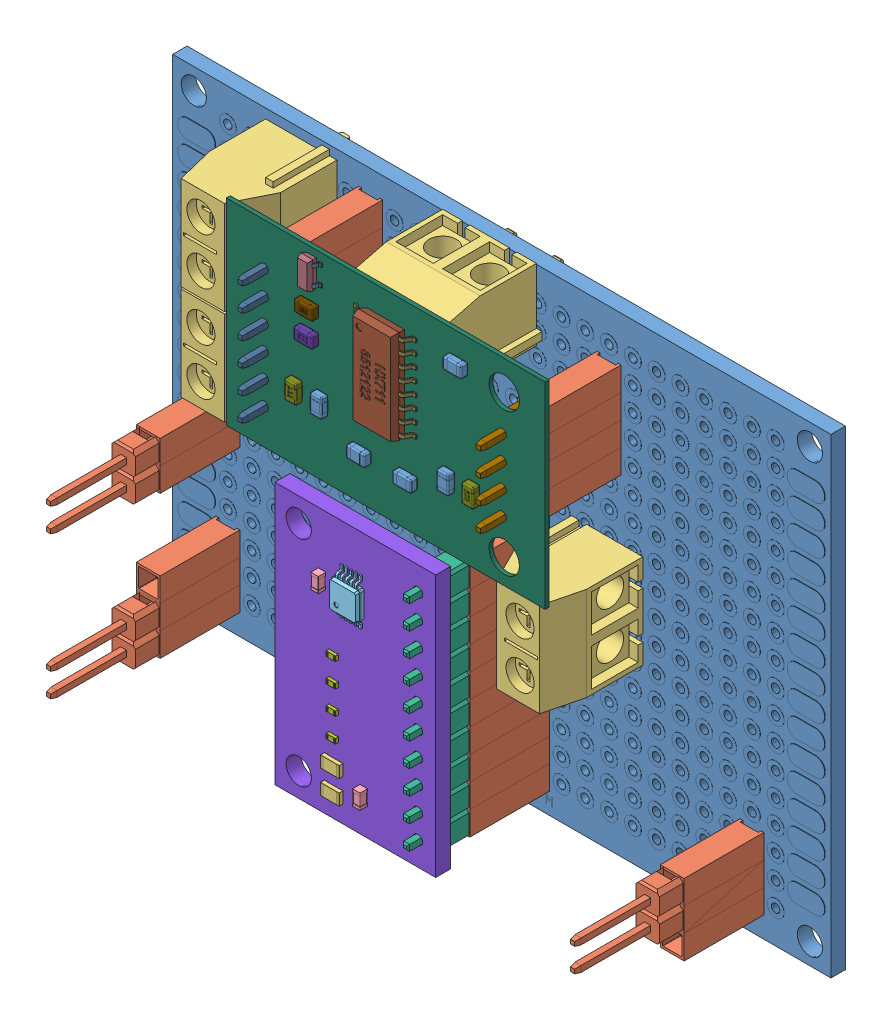
SolidWorks assembly ADCPCB, configuration Default. Lengths in mm.
Overall size (70.2 51.25 24.04).
104 component instances, 21 part files, 65 mates.
Components (placement in the parent):
- 5x7PCBBoard.stp-1: 5x7PCBBoard.stp [Default] at origin size (70.2 50.2 1.66)
- FemalePinHeader2By1.stp-1: FemalePinHeader2By1.stp [Default] at (-29.21 -21.59 1.54) x (0 1 0) z (0 0 1) size (5.08 2.54 11.7)
  - Female Pin Header 1x.stp-1: Female Pin Header 1x.stp [Default] at origin size (2.54 2.54 11.7)
  - Female Pin Header 1x.stp-2: Female Pin Header 1x.stp [Default] at (2.54 0 0) size (2.54 2.54 11.7)
- FemalePinHeader2By1.stp-2: FemalePinHeader2By1.stp [Default] at (-29.21 -6.35 1.54) x (0 1 0) z (0 0 1) size (5.08 2.54 11.7)
  - Female Pin Header 1x.stp-1: Female Pin Header 1x.stp [Default] at origin size (2.54 2.54 11.7)
  - Female Pin Header 1x.stp-2: Female Pin Header 1x.stp [Default] at (2.54 0 0) size (2.54 2.54 11.7)
- FemalePinHeader2By1.stp-3: FemalePinHeader2By1.stp [Default] at (-29.21 -19.05 1.54) x (0 1 0) z (0 0 1) size (5.08 2.54 11.7)
  - Female Pin Header 1x.stp-1: Female Pin Header 1x.stp [Default] at origin size (2.54 2.54 11.7)
  - Female Pin Header 1x.stp-2: Female Pin Header 1x.stp [Default] at (2.54 0 0) size (2.54 2.54 11.7)
- FemalePinHeader2By1.stp-4: FemalePinHeader2By1.stp [Default] at (26.67 -21.59 1.54) x (0 1 0) z (0 0 1) size (5.08 2.54 11.7)
  - Female Pin Header 1x.stp-1: Female Pin Header 1x.stp [Default] at origin size (2.54 2.54 11.7)
  - Female Pin Header 1x.stp-2: Female Pin Header 1x.stp [Default] at (2.54 0 0) size (2.54 2.54 11.7)
- FemalePinHeader2By1.stp-5: FemalePinHeader2By1.stp [Default] at (26.67 -19.05 1.54) x (0 1 0) z (0 0 1) size (5.08 2.54 11.7)
  - Female Pin Header 1x.stp-1: Female Pin Header 1x.stp [Default] at origin size (2.54 2.54 11.7)
  - Female Pin Header 1x.stp-2: Female Pin Header 1x.stp [Default] at (2.54 0 0) size (2.54 2.54 11.7)
- FemalePinHeader10By1.stp-1: FemalePinHeader10By1.stp [Default] at (3.81 1.27 1.54) x (0 -1 0) z (0 0 1) size (25.4 2.54 11.7)
  - Female Pin Header 1x.stp-1: Female Pin Header 1x.stp [Default] at origin size (2.54 2.54 11.7)
  - Female Pin Header 1x.stp-2: Female Pin Header 1x.stp [Default] at (2.54 0 0) size (2.54 2.54 11.7)
  - Female Pin Header 1x.stp-3: Female Pin Header 1x.stp [Default] at (5.08 0 0) size (2.54 2.54 11.7)
  - Female Pin Header 1x.stp-4: Female Pin Header 1x.stp [Default] at (7.62 0 0) size (2.54 2.54 11.7)
  - Female Pin Header 1x.stp-5: Female Pin Header 1x.stp [Default] at (10.16 0 0) size (2.54 2.54 11.7)
  - Female Pin Header 1x.stp-6: Female Pin Header 1x.stp [Default] at (12.7 0 0) size (2.54 2.54 11.7)
  - Female Pin Header 1x.stp-7: Female Pin Header 1x.stp [Default] at (15.24 0 0) size (2.54 2.54 11.7)
  - Female Pin Header 1x.stp-8: Female Pin Header 1x.stp [Default] at (17.78 0 0) size (2.54 2.54 11.7)
  - Female Pin Header 1x.stp-9: Female Pin Header 1x.stp [Default] at (20.32 0 0) size (2.54 2.54 11.7)
  - Female Pin Header 1x.stp-10: Female Pin Header 1x.stp [Default] at (22.86 0 0) size (2.54 2.54 11.7)
- FemalePinHeader6By1.stp-1: FemalePinHeader6By1.stp [Default] at (-13.97 21.59 1.54) x (0 -1 0) z (0 0 1) size (15.24 2.54 11.7)
  - Female Pin Header 1x.stp-1: Female Pin Header 1x.stp [Default] at origin size (2.54 2.54 11.7)
  - Female Pin Header 1x.stp-2: Female Pin Header 1x.stp [Default] at (2.54 0 0) size (2.54 2.54 11.7)
  - Female Pin Header 1x.stp-3: Female Pin Header 1x.stp [Default] at (5.08 0 0) size (2.54 2.54 11.7)
  - Female Pin Header 1x.stp-4: Female Pin Header 1x.stp [Default] at (7.62 0 0) size (2.54 2.54 11.7)
  - Female Pin Header 1x.stp-5: Female Pin Header 1x.stp [Default] at (10.16 0 0) size (2.54 2.54 11.7)
  - Female Pin Header 1x.stp-6: Female Pin Header 1x.stp [Default] at (12.7 0 0) size (2.54 2.54 11.7)
- FemalePinHeader4By1.stp-1: FemalePinHeader4By1.stp [Default] at (11.44 19.05 1.54) x (0 -1 0) z (0 0 1) size (10.16 2.54 11.7)
  - Female Pin Header 1x.stp-1: Female Pin Header 1x.stp [Default] at origin size (2.54 2.54 11.7)
  - Female Pin Header 1x.stp-2: Female Pin Header 1x.stp [Default] at (2.54 0 0) size (2.54 2.54 11.7)
  - Female Pin Header 1x.stp-3: Female Pin Header 1x.stp [Default] at (5.08 0 0) size (2.54 2.54 11.7)
  - Female Pin Header 1x.stp-4: Female Pin Header 1x.stp [Default] at (7.62 0 0) size (2.54 2.54 11.7)
- ADS1115+PinHeader.step-1: ADS1115+PinHeader.step [Default] at (144.065 -99.14 12.63) x (-1 0 0) z (0 0 1) size (17.14 27.94 11.54)
  - R_0805_2012Metric.step-1: R_0805_2012Metric.step [Default] at (149.225 -80.01 1.65) size (2 1.2 0.45)
    - SOLID.step-1: SOLID.step [Default] at origin size (2 1.2 0.45)
  - R_0805_2012Metric.step-2: R_0805_2012Metric.step [Default] at (149.225 -77.47 1.65) size (2 1.2 0.45)
    - SOLID.step-1: SOLID.step [Default] at origin size (2 1.2 0.45)
  - C_0603_1608Metric.step-1: C_0603_1608Metric.step [Default] at (150.495 -96.52 1.65) x (0 1 0) z (0 0 1) size (1.6 0.8 0.8)
    - SOLID-0.step-1: SOLID-0.step [Default] at origin size (1.6 0.8 0.8)
  - TSSOP-10_3x3mm_P0.5mm.step-1: TSSOP-10_3x3mm_P0.5mm.step [Default] at (147.32 -96.52 1.65) x (0 -1 0) z (0 0 1) size (4.9 3 1)
    - SOLID-1.step-1: SOLID-1.step [Default] at origin size (4.9 3 1)
  - PinHeader_1x10_P2.54mm_Vertical.step-1: PinHeader_1x10_P2.54mm_Vertical.step [Default] at (140.335 -77.47 -0.05) x (-1 0 0) z (0 0 -1) size (2.54 25.4 11.54)
    - SOLID-2.step-1: SOLID-2.step [Default] at origin size (2.54 25.4 11.54)
  - C_0603_1608Metric.step-2: C_0603_1608Metric.step [Default] at (146.05 -78.74 1.65) x (0 1 0) z (0 0 1) size (1.6 0.8 0.8)
    - SOLID-0.step-1: SOLID-0.step [Default] at origin size (1.6 0.8 0.8)
  - R_0402_1005Metric.step-1: R_0402_1005Metric.step [Default] at (149.225 -85.09 1.65) x (-1 0 0) z (0 0 1) size (1 0.5 0.35)
    - SOLID-3.step-1: SOLID-3.step [Default] at origin size (1 0.5 0.35)
  - R_0402_1005Metric.step-2: R_0402_1005Metric.step [Default] at (149.225 -82.55 1.65) x (-1 0 0) z (0 0 1) size (1 0.5 0.35)
    - SOLID-3.step-1: SOLID-3.step [Default] at origin size (1 0.5 0.35)
  - R_0402_1005Metric.step-3: R_0402_1005Metric.step [Default] at (149.225 -87.63 1.65) size (1 0.5 0.35)
    - SOLID-3.step-1: SOLID-3.step [Default] at origin size (1 0.5 0.35)
  - R_0402_1005Metric.step-4: R_0402_1005Metric.step [Default] at (149.225 -90.17 1.65) x (-1 0 0) z (0 0 1) size (1 0.5 0.35)
    - SOLID-3.step-1: SOLID-3.step [Default] at origin size (1 0.5 0.35)
  - COMPOUND.step-1: COMPOUND.step [Default] at origin size (17.14 27.94 1.6)
- 1x4 Male Pin Header.step-1: 1x4 Male Pin Header.step [Default] at (11.52 11.51 12.58) x (0 1 0) z (-1 0 0) size (10.17 13.54 2.5)
- 1x6 Male Pin Header.step-1: 1x6 Male Pin Header.step [Default] at (-13.89 8.97 12.58) x (0 1 0) z (-1 0 0) size (15.24 13.54 2.5)
- HX711.STEP-1: HX711.STEP [Default] at (-17.9207 5.1545 12.58) size (34 21 1.97)
  - HX711_SOP16_Valor predeterminado.STEP-1: HX711_SOP16_Valor predeterminado.STEP [Default] at (16.3915 14.4374 -9.5535) size (6.7 10 1.56)
    - base_HX711_Valor predeterminado.STEP-1: base_HX711_Valor predeterminado.STEP [Default] at (0.6189 -0.8581 10) size (4.4 10 1.52)
    - pino_HX711_Valor predeterminado.STEP-1: pino_HX711_Valor predeterminado.STEP [Default] at (-2.7311 3.5869 10.04) x (0 -1 0) z (-1 0 0) size (0.4 0.86 1.3)
    - pino_HX711_Valor predeterminado.STEP-2: pino_HX711_Valor predeterminado.STEP [Default] at (-2.7311 2.3169 10.04) x (0 -1 0) z (-1 0 0) size (0.4 0.86 1.3)
    - pino_HX711_Valor predeterminado.STEP-3: pino_HX711_Valor predeterminado.STEP [Default] at (-2.7311 1.0469 10.04) x (0 -1 0) z (-1 0 0) size (0.4 0.86 1.3)
    - pino_HX711_Valor predeterminado.STEP-4: pino_HX711_Valor predeterminado.STEP [Default] at (-2.7311 -0.2231 10.04) x (0 -1 0) z (-1 0 0) size (0.4 0.86 1.3)
    - pino_HX711_Valor predeterminado.STEP-5: pino_HX711_Valor predeterminado.STEP [Default] at (-2.7311 -1.4931 10.04) x (0 -1 0) z (-1 0 0) size (0.4 0.86 1.3)
    - pino_HX711_Valor predeterminado.STEP-6: pino_HX711_Valor predeterminado.STEP [Default] at (-2.7311 -2.7631 10.04) x (0 -1 0) z (-1 0 0) size (0.4 0.86 1.3)
    - pino_HX711_Valor predeterminado.STEP-7: pino_HX711_Valor predeterminado.STEP [Default] at (-2.7311 -4.0331 10.04) x (0 -1 0) z (-1 0 0) size (0.4 0.86 1.3)
    - pino_HX711_Valor predeterminado.STEP-8: pino_HX711_Valor predeterminado.STEP [Default] at (-2.7311 -5.3031 10.04) x (0 -1 0) z (-1 0 0) size (0.4 0.86 1.3)
    - pino_HX711_Valor predeterminado.STEP-9: pino_HX711_Valor predeterminado.STEP [Default] at (3.9689 3.5869 10.04) x (0 1 0) z (1 0 0) size (0.4 0.86 1.3)
    - pino_HX711_Valor predeterminado.STEP-10: pino_HX711_Valor predeterminado.STEP [Default] at (3.9689 2.3169 10.04) x (0 1 0) z (1 0 0) size (0.4 0.86 1.3)
    - pino_HX711_Valor predeterminado.STEP-11: pino_HX711_Valor predeterminado.STEP [Default] at (3.9689 1.0469 10.04) x (0 1 0) z (1 0 0) size (0.4 0.86 1.3)
    - pino_HX711_Valor predeterminado.STEP-12: pino_HX711_Valor predeterminado.STEP [Default] at (3.9689 -0.2231 10.04) x (0 1 0) z (1 0 0) size (0.4 0.86 1.3)
    - pino_HX711_Valor predeterminado.STEP-13: pino_HX711_Valor predeterminado.STEP [Default] at (3.9689 -1.4931 10.04) x (0 1 0) z (1 0 0) size (0.4 0.86 1.3)
    - pino_HX711_Valor predeterminado.STEP-14: pino_HX711_Valor predeterminado.STEP [Default] at (3.9689 -2.7631 10.04) x (0 1 0) z (1 0 0) size (0.4 0.86 1.3)
    - pino_HX711_Valor predeterminado.STEP-15: pino_HX711_Valor predeterminado.STEP [Default] at (3.9689 -4.0331 10.04) x (0 1 0) z (1 0 0) size (0.4 0.86 1.3)
    - pino_HX711_Valor predeterminado.STEP-16: pino_HX711_Valor predeterminado.STEP [Default] at (3.9689 -5.3031 10.04) x (0 1 0) z (1 0 0) size (0.4 0.86 1.3)
  - SOT23_Valor predeterminado.STEP-1: SOT23_Valor predeterminado.STEP [Default] at (9.1544 19.1355 -2.4535) x (-1 0 0) z (0 0 1) size (2.3 2.9 1.03)
    - TRANSISTOR_SOT23_Valor predeterminado.STEP-1: TRANSISTOR_SOT23_Valor predeterminado.STEP [Default] at (0.0204 0.1428 2.9) size (1.3 2.9 1)
    - PINO_SOT23_Valor predeterminado.STEP-1: PINO_SOT23_Valor predeterminado.STEP [Default] at (-1.1296 1.0928 2.94) x (0 -1 0) z (-1 0 0) size (0.4 0.61 0.65)
    - PINO_SOT23_Valor predeterminado.STEP-2: PINO_SOT23_Valor predeterminado.STEP [Default] at (-1.1296 -0.8072 2.94) x (0 -1 0) z (-1 0 0) size (0.4 0.61 0.65)
    - PINO_SOT23_Valor predeterminado.STEP-3: PINO_SOT23_Valor predeterminado.STEP [Default] at (1.1704 0.1428 2.94) x (0 1 0) z (1 0 0) size (0.4 0.61 0.65)
  - placa_Valor predeterminado.STEP-1: placa_Valor predeterminado.STEP [Default] at origin size (34 21 0.41)
  - RESISTOR_SMD_122_Valor predeterminado.STEP-1: RESISTOR_SMD_122_Valor predeterminado.STEP [Default] at (7.557 7.2289 0.4215) x (0 1 0) z (-1 0 0) size (2 0.82 1.27)
  - RESISTOR_SMD_122_Valor predeterminado.STEP-2: RESISTOR_SMD_122_Valor predeterminado.STEP [Default] at (26.4556 7.0756 0.4215) x (0 1 0) z (-1 0 0) size (2 0.82 1.27)
  - RESISTOR_SMD_822_Valor predeterminado.STEP-1: RESISTOR_SMD_822_Valor predeterminado.STEP [Default] at (8.9272 12.9039 0.4215) x (-1 0 0) z (0 -1 0) size (2 0.82 1.27)
  - RESISTOR_SMD_203_Valor predeterminado.STEP-1: RESISTOR_SMD_203_Valor predeterminado.STEP [Default] at (8.9446 15.4759 0.4215) x (-1 0 0) z (0 -1 0) size (2 0.82 1.27)
  - CAPACITOR_805_Valor predeterminado.STEP-1: CAPACITOR_805_Valor predeterminado.STEP [Default] at (14.517 4.7561 0.4215) x (1 0 0) z (0 1 0) size (2 0.8 1.27)
  - CAPACITOR_805_Valor predeterminado.STEP-2: CAPACITOR_805_Valor predeterminado.STEP [Default] at (24.8147 18.1011 0.4215) x (1 0 0) z (0 1 0) size (2 0.8 1.27)
  - CAPACITOR_805_Valor predeterminado.STEP-3: CAPACITOR_805_Valor predeterminado.STEP [Default] at (19.4533 4.8571 0.4215) x (1 0 0) z (0 1 0) size (2 0.8 1.27)
  - CAPACITOR_805_Valor predeterminado.STEP-4: CAPACITOR_805_Valor predeterminado.STEP [Default] at (23.7861 6.9684 0.4215) x (0 -1 0) z (1 0 0) size (2 0.8 1.27)
  - CAPACITOR_805_Valor predeterminado.STEP-5: CAPACITOR_805_Valor predeterminado.STEP [Default] at (10.279 7.2922 0.4215) x (0 -1 0) z (1 0 0) size (2 0.8 1.27)
- 1x2 Male Pin Header.step-1: 1x2 Male Pin Header.step [Default] at (-29.29 -19.13 10.04) x (0 -1 0) z (-1 0 0) size (5.08 13.54 2.5)
- 1x2 Male Pin Header.step-2: 1x2 Male Pin Header.step [Default] at (-29.29 -3.89 10.04) x (0 -1 0) z (-1 0 0) size (5.08 13.54 2.5)
- 1x2 Male Pin Header.step-3: 1x2 Male Pin Header.step [Default] at (26.59 -16.59 10.04) x (0 -1 0) z (-1 0 0) size (5.08 13.54 2.5)
- 5mm2PTerminalBlock-1: 5mm2PTerminalBlock [Default] at (-25.19 24.09 1.54) x (0 -1 0) z (0 0 1) size (10.6 7.6 15)
- 5mm2PTerminalBlock-2: 5mm2PTerminalBlock [Default] at (-25.19 13.89 1.54) x (0 -1 0) z (0 0 1) size (10.6 7.6 15)
- 5mm2PTerminalBlock-3: 5mm2PTerminalBlock [Default] at (3.69 25.19 1.54) x (-1 0 0) z (0 0 1) size (10.6 7.6 15)
- 5mm2PTerminalBlock-4: 5mm2PTerminalBlock [Default] at (15.04 -6.23 1.54) x (0 1 0) z (0 0 1) size (10.6 7.6 15)
Mates (geometry in assembly coordinates):
- Coincident1: coincident aligned: plane of 5x7PCBBoard.stp-1 through (0 0 0) normal (0 0 1)
- Coincident2: coincident aligned: plane of 5x7PCBBoard.stp-1 through (0 0 0) normal (0 1 0)
- Coincident3: coincident aligned: plane of 5x7PCBBoard.stp-1 through (0 0 0) normal (1 0 0)
- Parallel1: parallel anti-aligned: plane of 5x7PCBBoard.stp-1 through (-35.1 -25.1 0) normal (-1 0 0); plane of FemalePinHeader2By1.stp-1/Female Pin Header 1x.stp-2 through (-27.94 -20.32 1.54) normal (1 0 0)
- Parallel2: parallel aligned: plane of 5x7PCBBoard.stp-1 through (35.1 -25.1 0) normal (0 -1 0); plane of FemalePinHeader2By1.stp-1/Female Pin Header 1x.stp-1 through (-30.48 -22.86 1.54) normal (0 -1 0)
- Coincident6: coincident anti-aligned: plane of 5x7PCBBoard.stp-1 through (0 0 1.54) normal (0 0 1); plane of FemalePinHeader2By1.stp-1/Female Pin Header 1x.stp-1 through (-29.21 -21.59 1.54) normal (0 0 -1)
- Width1: width: plane of FemalePinHeader2By1.stp-1/Female Pin Header 1x.stp-1 through (-29.41 -20.49 1.54) normal (-1 0 0); plane of FemalePinHeader2By1.stp-1/Female Pin Header 1x.stp-1 through (-29.01 -22.69 1.54) normal (1 0 0); cylinder of 5x7PCBBoard.stp-1 through (-29.21 -21.59 0) axis (0 0 -1) radius 0.45
- Width2: width: plane of FemalePinHeader2By1.stp-1/Female Pin Header 1x.stp-1 through (-29.01 -21.915 2.34) normal (0 -1 0); plane of FemalePinHeader2By1.stp-1/Female Pin Header 1x.stp-1 through (-29.01 -21.265 -1.66) normal (0 1 0); cylinder of 5x7PCBBoard.stp-1 through (-29.2 -21.59 -0.005) axis (0 0 -1) radius 0.45
- Parallel4: parallel aligned: plane of 5x7PCBBoard.stp-1 through (35.1 -25.1 0) normal (0 -1 0); plane of FemalePinHeader10By1.stp-1/Female Pin Header 1x.stp-10 through (2.54 -22.86 1.54) normal (0 -1 0)
- Coincident10: coincident anti-aligned: plane of 5x7PCBBoard.stp-1 through (0 0 1.54) normal (0 0 1); plane of FemalePinHeader10By1.stp-1/Female Pin Header 1x.stp-10 through (3.81 -21.59 1.54) normal (0 0 -1)
- Parallel3: parallel aligned: plane of 5x7PCBBoard.stp-1 through (-35.1 -25.1 0) normal (-1 0 0); plane of FemalePinHeader10By1.stp-1/Female Pin Header 1x.stp-10 through (2.54 -20.32 1.54) normal (-1 0 0)
- Width3: width: plane of FemalePinHeader10By1.stp-1/Female Pin Header 1x.stp-10 through (3.61 -20.49 1.54) normal (-1 0 0); plane of FemalePinHeader10By1.stp-1/Female Pin Header 1x.stp-10 through (4.01 -22.69 1.54) normal (1 0 0); cylinder of 5x7PCBBoard.stp-1 through (3.81 -21.59 0) axis (0 0 -1) radius 0.45
- Width4: width: plane of FemalePinHeader10By1.stp-1/Female Pin Header 1x.stp-10 through (3.61 -21.915 -1.66) normal (0 -1 0); plane of FemalePinHeader10By1.stp-1/Female Pin Header 1x.stp-10 through (3.61 -21.265 2.34) normal (0 1 0); cylinder of 5x7PCBBoard.stp-1 through (3.81 -21.59 0) axis (0 0 -1) radius 0.45
- Parallel5: parallel aligned: plane of 5x7PCBBoard.stp-1 through (-35.1 25.1 0) normal (0 1 0); plane of FemalePinHeader6By1.stp-1/Female Pin Header 1x.stp-1 through (-12.7 22.86 1.54) normal (0 1 0)
- Parallel6: parallel aligned: plane of 5x7PCBBoard.stp-1 through (-35.1 -25.1 0) normal (-1 0 0); plane of FemalePinHeader6By1.stp-1/Female Pin Header 1x.stp-1 through (-15.24 22.86 1.54) normal (-1 0 0)
- Coincident14: coincident anti-aligned: plane of 5x7PCBBoard.stp-1 through (0 0 1.54) normal (0 0 1); plane of FemalePinHeader6By1.stp-1/Female Pin Header 1x.stp-1 through (-13.97 21.59 1.54) normal (0 0 -1)
- Width5: width: plane of FemalePinHeader6By1.stp-1/Female Pin Header 1x.stp-1 through (-14.17 22.69 1.54) normal (-1 0 0); plane of FemalePinHeader6By1.stp-1/Female Pin Header 1x.stp-1 through (-13.77 20.49 1.54) normal (1 0 0); cylinder of 5x7PCBBoard.stp-1 through (-13.97 21.59 0) axis (0 0 -1) radius 0.45
- Width6: width: plane of FemalePinHeader6By1.stp-1/Female Pin Header 1x.stp-1 through (-14.17 21.915 2.34) normal (0 1 0); plane of FemalePinHeader6By1.stp-1/Female Pin Header 1x.stp-1 through (-14.17 21.265 -1.66) normal (0 -1 0); cylinder of 5x7PCBBoard.stp-1 through (-13.97 21.59 0) axis (0 0 -1) radius 0.45
- Parallel7: parallel aligned: plane of 5x7PCBBoard.stp-1 through (-35.1 25.1 0) normal (0 1 0); plane of FemalePinHeader4By1.stp-1/Female Pin Header 1x.stp-1 through (12.71 20.32 1.54) normal (0 1 0)
- Parallel8: parallel aligned: plane of 5x7PCBBoard.stp-1 through (35.1 25.1 0) normal (1 0 0); plane of FemalePinHeader4By1.stp-1/Female Pin Header 1x.stp-1 through (12.71 17.78 1.54) normal (1 0 0)
- Coincident17: coincident anti-aligned: plane of 5x7PCBBoard.stp-1 through (0 0 1.54) normal (0 0 1); plane of FemalePinHeader4By1.stp-1/Female Pin Header 1x.stp-1 through (11.44 19.05 1.54) normal (0 0 -1)
- Width7: width: plane of FemalePinHeader4By1.stp-1/Female Pin Header 1x.stp-1 through (11.24 19.375 2.34) normal (0 1 0); plane of FemalePinHeader4By1.stp-1/Female Pin Header 1x.stp-1 through (11.24 18.725 -1.66) normal (0 -1 0); cylinder of 5x7PCBBoard.stp-1 through (11.43 19.05 0) axis (0 0 -1) radius 0.45
- Width8: width: plane of FemalePinHeader4By1.stp-1/Female Pin Header 1x.stp-1 through (11.24 20.15 1.54) normal (-1 0 0); plane of FemalePinHeader4By1.stp-1/Female Pin Header 1x.stp-1 through (11.64 17.95 1.54) normal (1 0 0); cylinder of 5x7PCBBoard.stp-1 through (11.44 21.59 -0.005) axis (0 0 -1) radius 0.45
- Coincident18: coincident anti-aligned: plane of FemalePinHeader10By1.stp-1/Female Pin Header 1x.stp-10 through (3.41 -21.99 10.04) normal (1 0 0); plane of ADS1115+PinHeader.step-1/PinHeader_1x10_P2.54mm_Vertical.step-1/SOLID-2.step-1 through (3.41 -21.35 15.58) normal (-1 0 0)
- Coincident19: coincident anti-aligned: plane of FemalePinHeader10By1.stp-1/Female Pin Header 1x.stp-10 through (3.81 -21.59 10.04) normal (0 0 1); plane of ADS1115+PinHeader.step-1/PinHeader_1x10_P2.54mm_Vertical.step-1/SOLID-2.step-1 through (3.73 -10.24 10.04) normal (0 0 -1)
- Coincident20: coincident anti-aligned: plane of FemalePinHeader10By1.stp-1/Female Pin Header 1x.stp-10 through (4.21 -21.99 10.04) normal (0 1 0); plane of ADS1115+PinHeader.step-1/PinHeader_1x10_P2.54mm_Vertical.step-1/SOLID-2.step-1 through (3.41 -21.99 15.58) normal (0 -1 0)
- Coincident21: coincident anti-aligned: plane of FemalePinHeader4By1.stp-1/Female Pin Header 1x.stp-1 through (11.44 19.05 10.04) normal (0 0 1); plane of 1x4 Male Pin Header.step-1 through (11.52 19.13 10.04) normal (0 0 -1)
- Coincident22: coincident anti-aligned: plane of FemalePinHeader4By1.stp-1/Female Pin Header 1x.stp-1 through (11.84 19.45 10.04) normal (-1 0 0); plane of 1x4 Male Pin Header.step-1 through (11.84 18.81 2.04) normal (1 0 0)
- Coincident23: coincident anti-aligned: plane of FemalePinHeader4By1.stp-1/Female Pin Header 1x.stp-1 through (11.04 19.45 10.04) normal (0 -1 0); plane of 1x4 Male Pin Header.step-1 through (11.2 19.45 2.04) normal (0 1 0)
- Parallel9: parallel aligned: plane of 5x7PCBBoard.stp-1 through (-35.1 25.1 0) normal (0 1 0); plane of HX711.STEP-1/placa_Valor predeterminado.STEP-1 through (16.0793 26.1545 12.58) normal (0 1 0)
- Coincident24: coincident anti-aligned: plane of FemalePinHeader6By1.stp-1/Female Pin Header 1x.stp-1 through (-13.97 21.59 10.04) normal (0 0 1); plane of 1x6 Male Pin Header.step-1 through (-13.89 21.67 10.04) normal (0 0 -1)
- Coincident25: coincident anti-aligned: plane of FemalePinHeader6By1.stp-1/Female Pin Header 1x.stp-1 through (-14.37 21.99 10.04) normal (0 -1 0); plane of 1x6 Male Pin Header.step-1 through (-14.21 21.99 2.04) normal (0 1 0)
- Coincident26: coincident anti-aligned: plane of FemalePinHeader6By1.stp-1/Female Pin Header 1x.stp-1 through (-13.57 21.99 10.04) normal (-1 0 0); plane of 1x6 Male Pin Header.step-1 through (-13.57 21.35 2.04) normal (1 0 0)
- Width9: width: plane of 1x6 Male Pin Header.step-1 through (-13.57 21.35 2.04) normal (1 0 0); plane of 1x6 Male Pin Header.step-1 through (-14.21 21.35 2.04) normal (-1 0 0); cylinder of HX711.STEP-1/placa_Valor predeterminado.STEP-1 through (-13.89 21.67 12.58) axis (0 0 1) radius 0.45
- Width10: width: plane of 1x6 Male Pin Header.step-1 through (-14.21 21.99 2.04) normal (0 1 0); plane of 1x6 Male Pin Header.step-1 through (-14.21 21.35 2.04) normal (0 -1 0); cylinder of HX711.STEP-1/placa_Valor predeterminado.STEP-1 through (-13.89 21.67 12.58) axis (0 0 1) radius 0.45
- Coincident27: coincident anti-aligned: plane of 1x6 Male Pin Header.step-1 through (-13.89 8.97 12.58) normal (0 0 1); plane of HX711.STEP-1/placa_Valor predeterminado.STEP-1 through (-17.9207 5.1545 12.58) normal (0 0 -1)
- Coincident28: coincident anti-aligned: plane of FemalePinHeader2By1.stp-1/Female Pin Header 1x.stp-1 through (-29.21 -21.59 10.04) normal (0 0 1); plane of 1x2 Male Pin Header.step-1 through (-29.29 -19.13 10.04) normal (0 0 -1)
- Coincident29: coincident anti-aligned: plane of FemalePinHeader2By1.stp-1/Female Pin Header 1x.stp-1 through (-29.61 -21.99 10.04) normal (1 0 0); plane of 1x2 Male Pin Header.step-1 through (-29.61 -21.35 20.58) normal (-1 0 0)
- Coincident30: coincident anti-aligned: plane of FemalePinHeader2By1.stp-1/Female Pin Header 1x.stp-1 through (-28.81 -21.99 10.04) normal (0 1 0); plane of 1x2 Male Pin Header.step-1 through (-29.61 -21.99 20.58) normal (0 -1 0)
- Coincident31: coincident anti-aligned: plane of FemalePinHeader2By1.stp-2/Female Pin Header 1x.stp-1 through (-29.21 -6.35 10.04) normal (0 0 1); plane of 1x2 Male Pin Header.step-2 through (-29.29 -3.89 10.04) normal (0 0 -1)
- Coincident32: coincident anti-aligned: plane of FemalePinHeader2By1.stp-2/Female Pin Header 1x.stp-1 through (-29.61 -6.75 10.04) normal (1 0 0); plane of 1x2 Male Pin Header.step-2 through (-29.61 -6.11 20.58) normal (-1 0 0)
- Coincident33: coincident anti-aligned: plane of FemalePinHeader2By1.stp-2/Female Pin Header 1x.stp-1 through (-28.81 -6.75 10.04) normal (0 1 0); plane of 1x2 Male Pin Header.step-2 through (-29.61 -6.75 20.58) normal (0 -1 0)
- Coincident34: coincident anti-aligned: plane of FemalePinHeader2By1.stp-4/Female Pin Header 1x.stp-2 through (26.67 -19.05 10.04) normal (0 0 1); plane of 1x2 Male Pin Header.step-3 through (26.59 -16.59 10.04) normal (0 0 -1)
- Coincident35: coincident anti-aligned: plane of FemalePinHeader2By1.stp-4/Female Pin Header 1x.stp-2 through (27.07 -19.45 10.04) normal (0 1 0); plane of 1x2 Male Pin Header.step-3 through (26.27 -19.45 20.58) normal (0 -1 0)
- Coincident36: coincident anti-aligned: plane of FemalePinHeader2By1.stp-4/Female Pin Header 1x.stp-2 through (26.27 -19.45 10.04) normal (1 0 0); plane of 1x2 Male Pin Header.step-3 through (26.27 -18.81 20.58) normal (-1 0 0)
- Parallel10: parallel aligned: plane of 5x7PCBBoard.stp-1 through (-35.1 -25.1 0) normal (-1 0 0); plane of 5mm2PTerminalBlock.step-1/Cut007.step-1 through (-25.18 24.09 1.54) normal (-1 0 0)
- Parallel11: parallel aligned: plane of 5x7PCBBoard.stp-1 through (-35.1 25.1 0) normal (0 1 0); plane of 5mm2PTerminalBlock.step-1/Cut007.step-1 through (-25.18 24.09 1.54) normal (0 1 0)
- Width11: width: plane of 5mm2PTerminalBlock.step-1/Patas.step-1/Fillet001.step-1 through (-21.08 21.99 -3.46) normal (1 0 0); plane of 5mm2PTerminalBlock.step-1/Patas.step-1/Fillet001.step-1 through (-22.08 21.99 -3.46) normal (-1 0 0); cylinder of 5x7PCBBoard.stp-1 through (-21.58 21.59 -0.005) axis (0 0 -1) radius 0.45
- Width12: width: plane of 5mm2PTerminalBlock.step-1/Patas.step-1/Fillet001.step-1 through (-22.08 21.99 -3.46) normal (0 1 0); plane of 5mm2PTerminalBlock.step-1/Patas.step-1/Fillet001.step-1 through (-22.08 21.19 -3.46) normal (0 -1 0); cylinder of 5x7PCBBoard.stp-1 through (-21.59 21.59 0) axis (0 0 -1) radius 0.45
- Coincident39: coincident anti-aligned: plane of 5x7PCBBoard.stp-1 through (0 0 1.54) normal (0 0 1); plane of 5mm2PTerminalBlock.step-1/Cut007.step-1 through (-25.18 24.09 1.54) normal (0 0 -1)
- Parallel13: parallel aligned: plane of 5x7PCBBoard.stp-1 through (-35.1 -25.1 0) normal (-1 0 0); plane of 5mm2PTerminalBlock-1 through (-25.19 24.09 1.54) normal (-1 0 0)
- Parallel12: parallel aligned: plane of 5x7PCBBoard.stp-1 through (-35.1 25.1 0) normal (0 1 0); plane of 5mm2PTerminalBlock-1 through (-25.19 24.09 1.54) normal (0 1 0)
- Coincident42: coincident anti-aligned: plane of 5x7PCBBoard.stp-1 through (0 0 1.54) normal (0 0 1); plane of 5mm2PTerminalBlock-1 through (-25.19 24.09 1.54) normal (0 0 -1)
- Width13: width: plane of 5mm2PTerminalBlock-1 through (-21.09 21.99 -3.46) normal (1 0 0); plane of 5mm2PTerminalBlock-1 through (-22.09 21.99 -3.46) normal (-1 0 0); cylinder of 5x7PCBBoard.stp-1 through (-21.59 21.59 0) axis (0 0 -1) radius 0.45
- Width14: width: plane of 5mm2PTerminalBlock-1 through (-22.09 21.99 -3.46) normal (0 1 0); plane of 5mm2PTerminalBlock-1 through (-22.09 21.19 -3.46) normal (0 -1 0); cylinder of 5x7PCBBoard.stp-1 through (-21.59 21.59 0) axis (0 0 -1) radius 0.45
- Parallel14: parallel anti-aligned: plane of 5x7PCBBoard.stp-1 through (-35.1 25.1 0) normal (0 1 0); plane of 5mm2PTerminalBlock-3 through (3.69 17.59 1.54) normal (0 -1 0)
- Coincident44: coincident anti-aligned: plane of 5x7PCBBoard.stp-1 through (0 0 1.54) normal (0 0 1); plane of 5mm2PTerminalBlock-3 through (3.69 25.19 1.54) normal (0 0 -1)
- Coincident45: coincident anti-aligned: plane of 5x7PCBBoard.stp-1 through (0 0 1.54) normal (0 0 1); plane of 5mm2PTerminalBlock-3 through (3.69 25.19 1.54) normal (0 0 -1)
- Width15: width: plane of 5mm2PTerminalBlock-3 through (-3.41 22.09 -3.46) normal (0 1 0); plane of 5mm2PTerminalBlock-3 through (-3.41 21.09 -3.46) normal (0 -1 0); cylinder of 5x7PCBBoard.stp-1 through (-3.81 21.59 0) axis (0 0 -1) radius 0.45
- Width16: width: plane of 5mm2PTerminalBlock-3 through (-3.41 22.09 -3.46) normal (1 0 0); plane of 5mm2PTerminalBlock-3 through (-4.21 22.09 -3.46) normal (-1 0 0); cylinder of 5x7PCBBoard.stp-1 through (-3.81 21.59 0) axis (0 0 -1) radius 0.45
- Parallel15: parallel aligned: plane of 5x7PCBBoard.stp-1 through (35.1 25.1 0) normal (1 0 0); plane of 5mm2PTerminalBlock-4 through (15.04 -6.23 1.54) normal (1 0 0)
- Coincident47: coincident anti-aligned: plane of 5x7PCBBoard.stp-1 through (0 0 1.54) normal (0 0 1); plane of 5mm2PTerminalBlock-4 through (15.04 -6.23 1.54) normal (0 0 -1)
- Parallel16: parallel aligned: plane of 5x7PCBBoard.stp-1 through (35.1 -25.1 0) normal (0 -1 0); plane of 5mm2PTerminalBlock-4 through (15.04 -6.23 1.54) normal (0 -1 0)
- Width17: width: plane of 5mm2PTerminalBlock-4 through (10.94 0.87 -3.46) normal (-1 0 0); plane of 5mm2PTerminalBlock-4 through (11.94 0.87 -3.46) normal (1 0 0); cylinder of 5x7PCBBoard.stp-1 through (11.44 1.27 -0.005) axis (0 0 -1) radius 0.45
- Width18: width: plane of 5mm2PTerminalBlock-4 through (11.94 0.87 -3.46) normal (0 -1 0); plane of 5mm2PTerminalBlock-4 through (11.94 1.67 -3.46) normal (0 1 0); cylinder of 5x7PCBBoard.stp-1 through (11.43 1.27 0) axis (0 0 -1) radius 0.45
